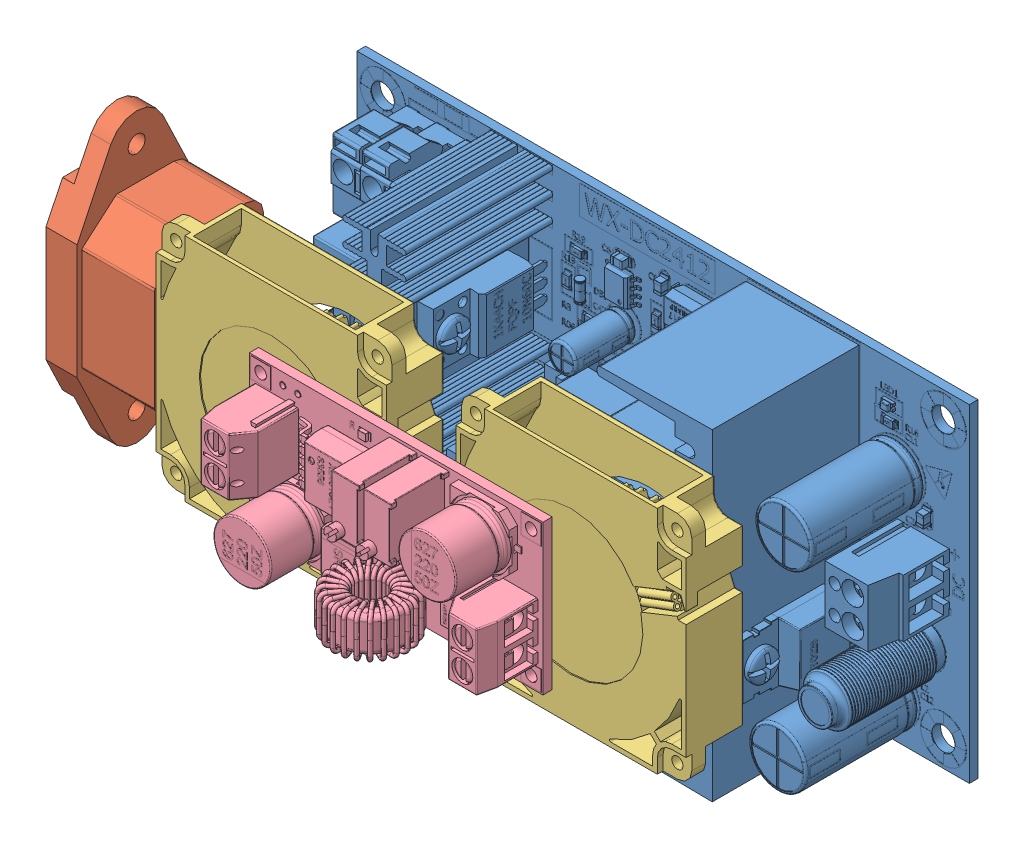
SolidWorks assembly Сборка8, configuration По умолчанию. Lengths in mm.
Overall size (125.8 57 70.27).
5 component instances, 4 part files, 2 mates.
Components (placement in the parent):
- WX-DC2412-1: WX-DC2412 [По умолчанию] at origin size (106.4 57 37.02)
- interlock.stp-1: interlock.stp [По умолчанию] at (-67.1973 -0.3307 25.7827) x (0 1 0) z (-1 0 0) size (50 20.7 27.56)
- 4010 turbo fan v3-1: 4010 turbo fan v3 [По умолчанию] at (-26.8704 6.9974 42.7223) x (0 -1 0) z (0 0 -1) size (40 40 10)
- 4010 turbo fan v3-2: 4010 turbo fan v3 [По умолчанию] at (25.201 6.9974 42.7223) x (0 -1 0) z (0 0 -1) size (40 40 10)
- XL4015 StepDown DC-DC 5A (CC-CV) v1-2: XL4015 StepDown DC-DC 5A (CC-CV) v1 [По умолчанию] at (-25.4878 -5.8352 46.3006) size (51 26 18.15)
Mates (geometry in assembly coordinates):
- Совпадение1: coincident aligned: plane of 4010 turbo fan v3-1 through (-26.8704 6.9974 42.7223) normal (0 0 1); plane of 4010 turbo fan v3-2 through (25.201 6.9974 42.7223) normal (0 0 1)
- Совпадение2: coincident aligned: plane of 4010 turbo fan v3-1 through (-41.8704 26.9974 42.7223) normal (0 1 0); plane of 4010 turbo fan v3-2 through (10.201 26.9974 42.7223) normal (0 1 0)
